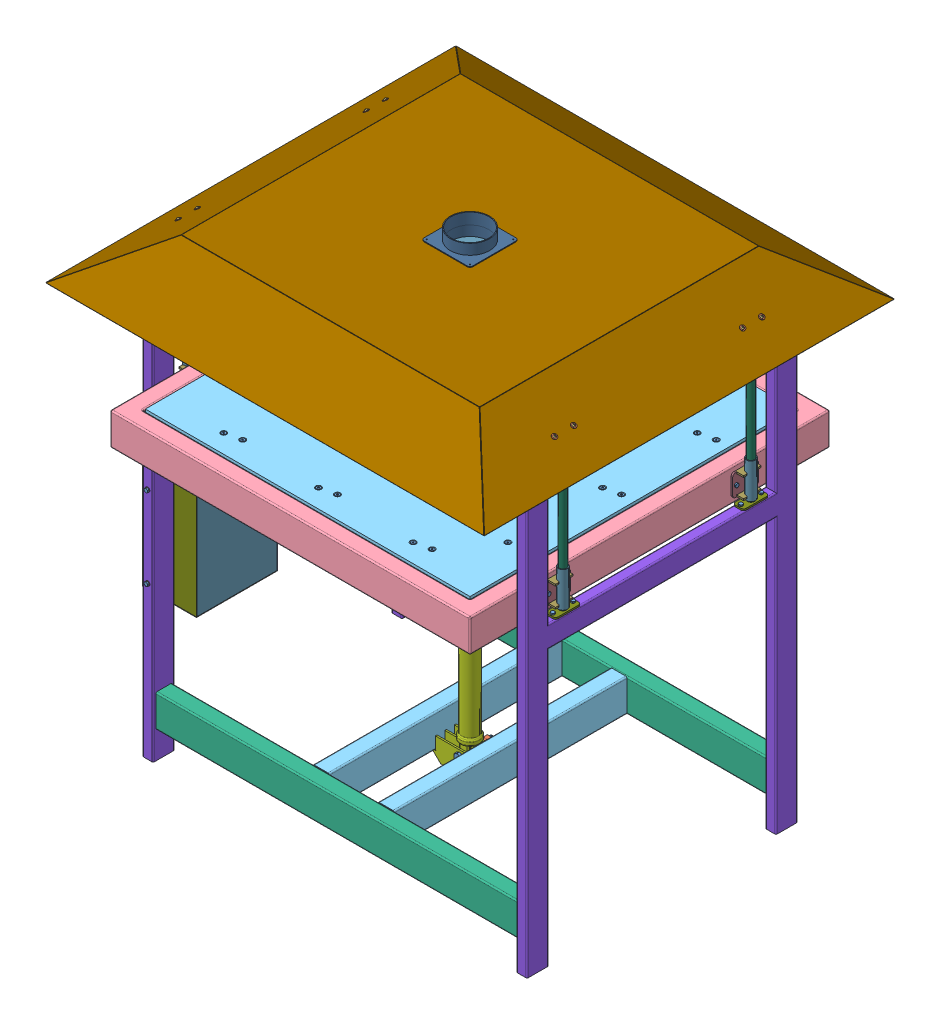
SolidWorks assembly SPR-V1 0000.00-A Sheetpress assembly, configuration Default. Lengths in mm.
Overall size (1624.97 1798.5 1807.96).
665 component instances, 57 part files, 108 mates.
Components (placement in the parent):
- hex bolt gradeab_iso-8: hex bolt gradeab_iso [ISO 4014 - M16 x 120 x 38-S] at (0 -1389 48) x (0 0 -1) z (1 0 0) size (130 27.71 24)
- hex bolt gradeab_iso-10: hex bolt gradeab_iso [ISO 4014 - M16 x 140 x 140-S] at (22.6273 -546.9999 22.6275) x (-0.707107 0 -0.707107) z (0.707107 0 -0.707107) size (150 27.71 24)
- hex nut gradec_iso-137: hex nut gradec_iso [ISO - 4034 - M16 - N] at (0 -1389 -69.8) x (0.923728 0.383049 0) z (0 0 -1) size (24 27.71 15.9)
- hex nut gradec_iso-140: hex nut gradec_iso [ISO - 4034 - M16 - N] at (-65.1246 -546.9999 -65.1245) x (-0.707107 0 0.707107) z (-0.707107 0 -0.707107) size (24 27.71 15.9)
- hex nut gradec_iso-141: hex nut gradec_iso [ISO - 4034 - M16 - N] at (-76.3676 -546.9999 -76.3675) x (-0.707085 -0.007759 0.707085) z (-0.707107 0 -0.707107) size (24 27.71 15.9)
- hex nut gradec_iso-136: hex nut gradec_iso [ISO - 4034 - M16 - N] at (0 -1389 -53.9) x (0.923728 0.383049 0) z (0 0 -1) size (24 27.71 15.9)
- SPR-V1 0000.03-A Spacer-1: SPR-V1 0000.03-A Spacer [Default] at (665 0 0) x (0 0 -1) z (1 0 0) size (40 40 6)
- SPR-V1 0000.03-A Spacer-2: SPR-V1 0000.03-A Spacer [Default] at (671 0 0) x (0 0 1) z (-1 0 0) size (40 40 6)
- SPR-V1 0000.03-A Spacer-3: SPR-V1 0000.03-A Spacer [Default] at (-671 0 0) x (0 0 -1) z (1 0 0) size (40 40 6)
- SPR-V1 0000.03-A Spacer-4: SPR-V1 0000.03-A Spacer [Default] at (-665 0 0) x (0 0 1) z (-1 0 0) size (40 40 6)
- SPR-V1 0000.03-A Spacer-5: SPR-V1 0000.03-A Spacer [Default] at (671 0 -350) x (0 0 1) z (-1 0 0) size (40 40 6)
- SPR-V1 0000.03-A Spacer-6: SPR-V1 0000.03-A Spacer [Default] at (-665 0 -350) x (0 0 1) z (-1 0 0) size (40 40 6)
- plain washer normal grade a_iso-1: plain washer normal grade a_iso [Washer ISO 7089 - 16] at (-711 80 350) size (3 30 30)
- plain washer normal grade a_iso-2: plain washer normal grade a_iso [Washer ISO 7089 - 16] at (-711 80 0) size (3 30 30)
- plain washer normal grade a_iso-3: plain washer normal grade a_iso [Washer ISO 7089 - 16] at (-711 80 -350) size (3 30 30)
- plain washer normal grade a_iso-4: plain washer normal grade a_iso [Washer ISO 7089 - 16] at (605 80 350) size (3 30 30)
- plain washer normal grade a_iso-5: plain washer normal grade a_iso [Washer ISO 7089 - 16] at (605 80 0) size (3 30 30)
- plain washer normal grade a_iso-6: plain washer normal grade a_iso [Washer ISO 7089 - 16] at (605 80 -350) size (3 30 30)
- plain washer normal grade a_iso-7: plain washer normal grade a_iso [Washer ISO 7089 - 16] at (711 80 350) x (-1 0 0) z (0 0.924225 0.381849) size (3 30 30)
- plain washer normal grade a_iso-8: plain washer normal grade a_iso [Washer ISO 7089 - 16] at (711 80 0) x (-1 0 0) z (0 0.924225 0.381849) size (3 30 30)
- plain washer normal grade a_iso-9: plain washer normal grade a_iso [Washer ISO 7089 - 16] at (711 80 -350) x (-1 0 0) z (0 0.924225 0.381849) size (3 30 30)
- plain washer normal grade a_iso-10: plain washer normal grade a_iso [Washer ISO 7089 - 16] at (-605 80 350) x (-1 0 0) z (0 0.924225 0.381849) size (3 30 30)
- plain washer normal grade a_iso-11: plain washer normal grade a_iso [Washer ISO 7089 - 16] at (-605 80 0) x (-1 0 0) z (0 0.924225 0.381849) size (3 30 30)
- plain washer normal grade a_iso-12: plain washer normal grade a_iso [Washer ISO 7089 - 16] at (-605 80 -350) x (-1 0 0) z (0 0.924225 0.381849) size (3 30 30)
- hex bolt gradeab_iso-1: hex bolt gradeab_iso [ISO 4014 - M16 x 140 x 140-S] at (-724 80 350) size (150 27.71 24)
- hex bolt gradeab_iso-2: hex bolt gradeab_iso [ISO 4014 - M16 x 140 x 140-S] at (-724 80 -350) size (150 27.71 24)
- hex bolt gradeab_iso-3: hex bolt gradeab_iso [ISO 4014 - M16 x 140 x 140-S] at (-724 80 0) size (150 27.71 24)
- hex bolt gradeab_iso-4: hex bolt gradeab_iso [ISO 4014 - M16 x 140 x 140-S] at (724 80 -350) x (-1 0 0) z (0 0.924225 0.381849) size (150 27.71 24)
- hex bolt gradeab_iso-5: hex bolt gradeab_iso [ISO 4014 - M16 x 140 x 140-S] at (724 80 0) x (-1 0 0) z (0 0.924225 0.381849) size (150 27.71 24)
- hex bolt gradeab_iso-6: hex bolt gradeab_iso [ISO 4014 - M16 x 140 x 140-S] at (724 80 350) x (-1 0 0) z (0 0.924225 0.381849) size (150 27.71 24)
- hex nut gradec_iso-130: hex nut gradec_iso [ISO - 4034 - M16 - N] at (-586.1 80 -350) x (0 0 -1) z (1 0 0) size (24 27.71 15.9)
- hex nut gradec_iso-131: hex nut gradec_iso [ISO - 4034 - M8 - S] at (-594.1 80 0) x (0 0 -1) z (1 0 0) size (13 15.01 7.9)
- hex nut gradec_iso-132: hex nut gradec_iso [ISO - 4034 - M16 - N] at (-586.1 80 350) x (0 0 -1) z (1 0 0) size (24 27.71 15.9)
- hex nut gradec_iso-133: hex nut gradec_iso [ISO - 4034 - M16 - N] at (586.1 80 350) x (0 0 1) z (-1 0 0) size (24 27.71 15.9)
- hex nut gradec_iso-134: hex nut gradec_iso [ISO - 4034 - M16 - N] at (586.1 80 -350) x (0 0 1) z (-1 0 0) size (24 27.71 15.9)
- hex nut gradec_iso-135: hex nut gradec_iso [ISO - 4034 - M8 - S] at (594.1 80 0) x (0 0 1) z (-1 0 0) size (13 15.01 7.9)
- Frame^SPR-V1 0000.00-A Sheetpress assembly-1: Frame^SPR-V1 0000.00-A Sheetpress assembly [Default] at origin size (1422 1634 1000) (virtual)
  - SPR-V1 0000.01-A Bottom frame jack beams-1: SPR-V1 0000.01-A Bottom frame jack beams [Default] at origin size (300 120 860)
  - SPR-V1 0000.01-A Bottom Frame side beams-1: SPR-V1 0000.01-A Bottom Frame side beams [Default] at (0 0 430) size (1342 120 980)
  - SPR-V1 0000.01-A Jack mount lower-1: SPR-V1 0000.01-A Jack mount lower [Default] at (0 0 35) size (200 80 6)
  - SPR-V1 1000.01-A Side frame-1: SPR-V1 1000.01-A Side frame [Default] at (671 0 0) x (0 0 -1) z (1 0 0) size (1000 1634 40)
  - SPR-V1 1000.01-A Side frame-2: SPR-V1 1000.01-A Side frame [Default] at (-711 0 0) x (0 0 -1) z (1 0 0) size (1000 1634 40)
  - SPR-V1 0000.01-A Jack mount lower-2: SPR-V1 0000.01-A Jack mount lower [Default] at (0 0 -35) size (200 80 6)
  - SPR-V1 0000.01-A Jack mount lower-3: SPR-V1 0000.01-A Jack mount lower [Default] at origin size (200 80 6)
- Pressing plate upper^SPR-V1 0000.00-A Sheetpress assembly-2: Pressing plate upper^SPR-V1 0000.00-A Sheetpress assembly [Default] at origin size (1356.27 127.4 1715) (virtual)
  - SPR-V1 2100.01-A Pressing plate frame upper-1: SPR-V1 2100.01-A Pressing plate frame upper [Default] at origin size (1330 120 1330)
  - SPR-V1 2100.02-A Heating plate upper-1: SPR-V1 2100.02-A Heating plate upper [Default] x (-1 0 0) z (0 -1 0) size (1200 1200 10)
  - SPR-V1 2100.03-A Support structure upper B-1: SPR-V1 2100.03-A Support structure upper B [Default] at (0 107 0) x (-1 0 0) z (0 0 1) size (1210 100 1210)
  - SPR-V1 2100.03-A Pressing plate support structure upper A-1: SPR-V1 2100.03-A Pressing plate support structure upper A [Default] at (0 7 0) size (1210 100 1210)
  - SPR-V1 2100.04-A Sheet mount tabs upper-1: SPR-V1 2100.04-A Sheet mount tabs upper [Default] at (0 118 0) x (-1 0 0) z (0 -1 0) size (46.67 46.67 6.35)
  - SPR-V1 2000.01-A Sheet cover upper-1: SPR-V1 2000.01-A Sheet cover upper [Default] at (0 112 0) x (1 0 0) z (0 1 0) size (1205 1205 1.5)
  - SPR-V1 2100.05-A Suspension plates-1: SPR-V1 2100.05-A Suspension plates [Default] at (260.3787 7 -260.3787) x (0.707107 0 0.707107) z (-0.707107 0 0.707107) size (50 6.43 86)
  - SPR-V1 12 Ceramic terminal-1: SPR-V1 12 Ceramic terminal [Default] at (89.6213 81 89.6213) x (0 -1 0) z (-0.707107 0 0.707107) size (52 24 30)
  - SPR-V1 14 M25 Cable Gland-1: SPR-V1 14 M25 Cable Gland [M20] at (-647.6252 59.9997 552.5039) x (0 0.998679 -0.05138) z (0 0.05138 0.998679) size (33.12 53.02 29.38)
  - SPR-V1 2100.05-A Suspension plates-2: SPR-V1 2100.05-A Suspension plates [Default] at (-260.3787 7 -260.3787) x (0.707107 0 -0.707107) z (0.707107 0 0.707107) size (50 6.43 86)
  - SPR-V1 2100.05-A Suspension plates-3: SPR-V1 2100.05-A Suspension plates [Default] at (-260.3787 7 260.3787) x (-0.707107 0 -0.707107) z (0.707107 0 -0.707107) size (50 6.43 86)
  - SPR-V1 2100.05-A Suspension plates-4: SPR-V1 2100.05-A Suspension plates [Default] at (260.3787 7 260.3787) x (-0.707107 0 0.707107) z (-0.707107 0 -0.707107) size (50 6.43 86)
  - SPR-V1 2000.02-A Heating block-35: SPR-V1 2000.02-A Heating block [Default] at (525.0056 7 524.9944) x (0.707107 0 -0.707107) z (0.707107 0 0.707107) size (50 25 80)
  - SPR-V1 2000.02-A Heating block-32: SPR-V1 2000.02-A Heating block [Default] at (175.0019 7 524.9944) x (0.707107 0 -0.707107) z (0.707107 0 0.707107) size (50 25 80)
  - SPR-V1 2000.02-A Heating block-33: SPR-V1 2000.02-A Heating block [Default] at (350.0037 7 349.9926) x (0.707107 0 -0.707107) z (0.707107 0 0.707107) size (50 25 80)
  - SPR-V1 2000.02-A Heating block-34: SPR-V1 2000.02-A Heating block [Default] at (525.0056 7 174.9907) x (0.707107 0 -0.707107) z (0.707107 0 0.707107) size (50 25 80)
  - SPR-V1 2000.02-A Heating block-44: SPR-V1 2000.02-A Heating block [Default] at (-175.0019 7 524.9944) x (0.707107 0 -0.707107) z (0.707107 0 0.707107) size (50 25 80)
  - SPR-V1 2000.02-A Heating block-45: SPR-V1 2000.02-A Heating block [Default] at (0 7 349.9926) x (0.707107 0 -0.707107) z (0.707107 0 0.707107) size (50 25 80)
  - SPR-V1 2000.02-A Heating block-46: SPR-V1 2000.02-A Heating block [Default] at (175.0019 7 174.9907) x (0.707107 0 -0.707107) z (0.707107 0 0.707107) size (50 25 80)
  - SPR-V1 2000.02-A Heating block-47: SPR-V1 2000.02-A Heating block [Default] at (350.0037 7 -0.0111) x (0.707107 0 -0.707107) z (0.707107 0 0.707107) size (50 25 80)
  - SPR-V1 2000.02-A Heating block-43: SPR-V1 2000.02-A Heating block [Default] at (525.0056 7 -175.013) x (0.707107 0 -0.707107) z (0.707107 0 0.707107) size (50 25 80)
  - SPR-V1 2000.02-A Heating block-36: SPR-V1 2000.02-A Heating block [Default] at (-525.0056 7 524.9944) x (0.707107 0 -0.707107) z (0.707107 0 0.707107) size (50 25 80)
  - SPR-V1 2000.02-A Heating block-37: SPR-V1 2000.02-A Heating block [Default] at (-350.0037 7 349.9926) x (0.707107 0 -0.707107) z (0.707107 0 0.707107) size (50 25 80)
  - SPR-V1 2000.02-A Heating block-42: SPR-V1 2000.02-A Heating block [Default] at (-175.0019 7 174.9907) x (0.707107 0 -0.707107) z (0.707107 0 0.707107) size (50 25 80)
  - SPR-V1 2000.02-A Heating block-38: SPR-V1 2000.02-A Heating block [Default] at (0 7 -0.0111) x (0.707107 0 -0.707107) z (0.707107 0 0.707107) size (50 25 80)
  - SPR-V1 2000.02-A Heating block-40: SPR-V1 2000.02-A Heating block [Default] at (175.0019 7 -175.013) x (0.707107 0 -0.707107) z (0.707107 0 0.707107) size (50 25 80)
  - SPR-V1 2000.02-A Heating block-39: SPR-V1 2000.02-A Heating block [Default] at (350.0037 7 -350.0149) x (0.707107 0 -0.707107) z (0.707107 0 0.707107) size (50 25 80)
  - SPR-V1 2000.02-A Heating block-41: SPR-V1 2000.02-A Heating block [Default] at (525.0056 7 -525.0167) x (0.707107 0 -0.707107) z (0.707107 0 0.707107) size (50 25 80)
  - SPR-V1 2000.02-A Heating block-26: SPR-V1 2000.02-A Heating block [Default] at (-525.0056 7 174.9907) x (0.707107 0 -0.707107) z (0.707107 0 0.707107) size (50 25 80)
  - SPR-V1 2000.02-A Heating block-24: SPR-V1 2000.02-A Heating block [Default] at (-350.0037 7 -0.0111) x (0.707107 0 -0.707107) z (0.707107 0 0.707107) size (50 25 80)
  - SPR-V1 2000.02-A Heating block-27: SPR-V1 2000.02-A Heating block [Default] at (-175.0019 7 -175.013) x (0.707107 0 -0.707107) z (0.707107 0 0.707107) size (50 25 80)
  - SPR-V1 2000.02-A Heating block-29: SPR-V1 2000.02-A Heating block [Default] at (0 7 -350.0149) x (0.707107 0 -0.707107) z (0.707107 0 0.707107) size (50 25 80)
  - SPR-V1 2000.02-A Heating block-30: SPR-V1 2000.02-A Heating block [Default] at (175.0019 7 -525.0167) x (0.707107 0 -0.707107) z (0.707107 0 0.707107) size (50 25 80)
  - SPR-V1 2000.02-A Heating block-31: SPR-V1 2000.02-A Heating block [Default] at (-525.0056 7 -175.013) x (0.707107 0 -0.707107) z (0.707107 0 0.707107) size (50 25 80)
  - SPR-V1 2000.02-A Heating block-23: SPR-V1 2000.02-A Heating block [Default] at (-350.0037 7 -350.0149) x (0.707107 0 -0.707107) z (0.707107 0 0.707107) size (50 25 80)
  - SPR-V1 2000.02-A Heating block-28: SPR-V1 2000.02-A Heating block [Default] at (-175.0019 7 -525.0167) x (0.707107 0 -0.707107) z (0.707107 0 0.707107) size (50 25 80)
  - SPR-V1 2000.02-A Heating block-25: SPR-V1 2000.02-A Heating block [Default] at (-525.0056 7 -525.0167) x (0.707107 0 -0.707107) z (0.707107 0 0.707107) size (50 25 80)
  - SPR-V1 12 Ceramic terminal-2: SPR-V1 12 Ceramic terminal [Default] at (89.6213 81 -89.6213) x (0 -1 0) z (0.707107 0 0.707107) size (52 24 30)
  - SPR-V1 12 Ceramic terminal-3: SPR-V1 12 Ceramic terminal [Default] at (-89.6213 81 -89.6213) x (0 -1 0) z (0.707107 0 -0.707107) size (52 24 30)
  - SPR-V1 12 Ceramic terminal-4: SPR-V1 12 Ceramic terminal [Default] at (-89.6213 81 89.6213) x (0 -1 0) z (-0.707107 0 -0.707107) size (52 24 30)
  - SPR-V1 2100.04-A Sheet mount tabs upper-2: SPR-V1 2100.04-A Sheet mount tabs upper [Default] at (0 118 0) x (0 0 1) z (0 -1 0) size (46.67 46.67 6.35)
  - SPR-V1 2100.04-A Sheet mount tabs upper-3: SPR-V1 2100.04-A Sheet mount tabs upper [Default] at (0 118 0) x (1 0 0) z (0 -1 0) size (46.67 46.67 6.35)
  - SPR-V1 2100.04-A Sheet mount tabs upper-4: SPR-V1 2100.04-A Sheet mount tabs upper [Default] at (0 118 0) x (0 0 -1) z (0 -1 0) size (46.67 46.67 6.35)
  - socket countersunk head screw_iso-1: socket countersunk head screw_iso [ISO 10642 - M8 x 50 - 28N] at (-531.5817 -3 -553.5131) x (0 1 0) z (0 0 1) size (50 15.24 15.24)
  - socket countersunk head screw_iso-2: socket countersunk head screw_iso [ISO 10642 - M8 x 50 - 28N] at (-181.578 -3 -553.5131) x (0 1 0) z (0 0 1) size (50 15.24 15.24)
  - socket countersunk head screw_iso-3: socket countersunk head screw_iso [ISO 10642 - M8 x 50 - 28N] at (-356.5798 -3 -378.5113) x (0 1 0) z (0 0 1) size (50 15.24 15.24)
  - socket countersunk head screw_iso-4: socket countersunk head screw_iso [ISO 10642 - M8 x 50 - 28N] at (-531.5817 -3 -203.5094) x (0 1 0) z (0 0 1) size (50 15.24 15.24)
  - socket countersunk head screw_iso-5: socket countersunk head screw_iso [ISO 10642 - M8 x 50 - 28N] at (168.4258 -3 -553.5131) x (0 1 0) z (0 0 1) size (50 15.24 15.24)
  - socket countersunk head screw_iso-6: socket countersunk head screw_iso [ISO 10642 - M8 x 50 - 28N] at (-6.5761 -3 -378.5113) x (0 1 0) z (0 0 1) size (50 15.24 15.24)
  - socket countersunk head screw_iso-7: socket countersunk head screw_iso [ISO 10642 - M8 x 50 - 28N] at (-181.578 -3 -203.5094) x (0 1 0) z (0 0 1) size (50 15.24 15.24)
  - socket countersunk head screw_iso-8: socket countersunk head screw_iso [ISO 10642 - M8 x 50 - 28N] at (-356.5798 -3 -28.5075) x (0 1 0) z (0 0 1) size (50 15.24 15.24)
  - socket countersunk head screw_iso-9: socket countersunk head screw_iso [ISO 10642 - M8 x 50 - 28N] at (-531.5817 -3 146.4943) x (0 1 0) z (0 0 1) size (50 15.24 15.24)
  - socket countersunk head screw_iso-10: socket countersunk head screw_iso [ISO 10642 - M8 x 50 - 28N] at (518.4295 -3 -553.5131) x (0 1 0) z (0 0 1) size (50 15.24 15.24)
  - socket countersunk head screw_iso-11: socket countersunk head screw_iso [ISO 10642 - M8 x 50 - 28N] at (343.4276 -3 -378.5113) x (0 1 0) z (0 0 1) size (50 15.24 15.24)
  - socket countersunk head screw_iso-12: socket countersunk head screw_iso [ISO 10642 - M8 x 50 - 28N] at (168.4258 -3 -203.5094) x (0 1 0) z (0 0 1) size (50 15.24 15.24)
  - socket countersunk head screw_iso-13: socket countersunk head screw_iso [ISO 10642 - M8 x 50 - 28N] at (-6.5761 -3 -28.5075) x (0 1 0) z (0 0 1) size (50 15.24 15.24)
  - socket countersunk head screw_iso-14: socket countersunk head screw_iso [ISO 10642 - M8 x 50 - 28N] at (-181.578 -3 146.4943) x (0 1 0) z (0 0 1) size (50 15.24 15.24)
  - socket countersunk head screw_iso-15: socket countersunk head screw_iso [ISO 10642 - M8 x 50 - 28N] at (-356.5798 -3 321.4962) x (0 1 0) z (0 0 1) size (50 15.24 15.24)
  - socket countersunk head screw_iso-16: socket countersunk head screw_iso [ISO 10642 - M8 x 50 - 28N] at (-531.5817 -3 496.498) x (0 1 0) z (0 0 1) size (50 15.24 15.24)
  - socket countersunk head screw_iso-17: socket countersunk head screw_iso [ISO 10642 - M8 x 50 - 28N] at (518.4295 -3 -203.5094) x (0 1 0) z (0 0 1) size (50 15.24 15.24)
  - socket countersunk head screw_iso-18: socket countersunk head screw_iso [ISO 10642 - M8 x 50 - 28N] at (343.4276 -3 -28.5075) x (0 1 0) z (0 0 1) size (50 15.24 15.24)
  - socket countersunk head screw_iso-19: socket countersunk head screw_iso [ISO 10642 - M8 x 50 - 28N] at (168.4258 -3 146.4943) x (0 1 0) z (0 0 1) size (50 15.24 15.24)
  - socket countersunk head screw_iso-20: socket countersunk head screw_iso [ISO 10642 - M8 x 50 - 28N] at (-6.5761 -3 321.4962) x (0 1 0) z (0 0 1) size (50 15.24 15.24)
  - socket countersunk head screw_iso-21: socket countersunk head screw_iso [ISO 10642 - M8 x 50 - 28N] at (-181.578 -3 496.498) x (0 1 0) z (0 0 1) size (50 15.24 15.24)
  - socket countersunk head screw_iso-22: socket countersunk head screw_iso [ISO 10642 - M8 x 50 - 28N] at (518.4295 -3 146.4943) x (0 1 0) z (0 0 1) size (50 15.24 15.24)
  - socket countersunk head screw_iso-23: socket countersunk head screw_iso [ISO 10642 - M8 x 50 - 28N] at (343.4276 -3 321.4962) x (0 1 0) z (0 0 1) size (50 15.24 15.24)
  - socket countersunk head screw_iso-24: socket countersunk head screw_iso [ISO 10642 - M8 x 50 - 28N] at (168.4258 -3 496.498) x (0 1 0) z (0 0 1) size (50 15.24 15.24)
  - socket countersunk head screw_iso-25: socket countersunk head screw_iso [ISO 10642 - M8 x 50 - 28N] at (518.4295 -3 496.498) x (0 1 0) z (0 0 1) size (50 15.24 15.24)
  - socket countersunk head screw_iso-26: socket countersunk head screw_iso [ISO 10642 - M8 x 50 - 28N] at (-518.4295 -3 -496.5203) x (0 1 0) z (-0.546944 0 0.837169) size (50 15.24 15.24)
  - socket countersunk head screw_iso-27: socket countersunk head screw_iso [ISO 10642 - M8 x 50 - 28N] at (-168.4258 -3 -496.5203) x (0 1 0) z (-0.546944 0 0.837169) size (50 15.24 15.24)
  - socket countersunk head screw_iso-28: socket countersunk head screw_iso [ISO 10642 - M8 x 50 - 28N] at (-343.4276 -3 -321.5185) x (0 1 0) z (-0.546944 0 0.837169) size (50 15.24 15.24)
  - socket countersunk head screw_iso-29: socket countersunk head screw_iso [ISO 10642 - M8 x 50 - 28N] at (-518.4295 -3 -146.5166) x (0 1 0) z (-0.546944 0 0.837169) size (50 15.24 15.24)
  - socket countersunk head screw_iso-30: socket countersunk head screw_iso [ISO 10642 - M8 x 50 - 28N] at (181.578 -3 -496.5203) x (0 1 0) z (-0.546944 0 0.837169) size (50 15.24 15.24)
  - socket countersunk head screw_iso-31: socket countersunk head screw_iso [ISO 10642 - M8 x 50 - 28N] at (6.5761 -3 -321.5185) x (0 1 0) z (-0.546944 0 0.837169) size (50 15.24 15.24)
  - socket countersunk head screw_iso-32: socket countersunk head screw_iso [ISO 10642 - M8 x 50 - 28N] at (-168.4258 -3 -146.5166) x (0 1 0) z (-0.546944 0 0.837169) size (50 15.24 15.24)
  - socket countersunk head screw_iso-33: socket countersunk head screw_iso [ISO 10642 - M8 x 50 - 28N] at (-343.4276 -3 28.4853) x (0 1 0) z (-0.546944 0 0.837169) size (50 15.24 15.24)
  - socket countersunk head screw_iso-34: socket countersunk head screw_iso [ISO 10642 - M8 x 50 - 28N] at (-518.4295 -3 203.4871) x (0 1 0) z (-0.546944 0 0.837169) size (50 15.24 15.24)
  - socket countersunk head screw_iso-35: socket countersunk head screw_iso [ISO 10642 - M8 x 50 - 28N] at (531.5817 -3 -496.5203) x (0 1 0) z (-0.546944 0 0.837169) size (50 15.24 15.24)
  - socket countersunk head screw_iso-36: socket countersunk head screw_iso [ISO 10642 - M8 x 50 - 28N] at (356.5798 -3 -321.5185) x (0 1 0) z (-0.546944 0 0.837169) size (50 15.24 15.24)
  - socket countersunk head screw_iso-37: socket countersunk head screw_iso [ISO 10642 - M8 x 50 - 28N] at (181.578 -3 -146.5166) x (0 1 0) z (-0.546944 0 0.837169) size (50 15.24 15.24)
  - socket countersunk head screw_iso-38: socket countersunk head screw_iso [ISO 10642 - M8 x 50 - 28N] at (6.5761 -3 28.4853) x (0 1 0) z (-0.546944 0 0.837169) size (50 15.24 15.24)
  - socket countersunk head screw_iso-39: socket countersunk head screw_iso [ISO 10642 - M8 x 50 - 28N] at (-168.4258 -3 203.4871) x (0 1 0) z (-0.546944 0 0.837169) size (50 15.24 15.24)
  - socket countersunk head screw_iso-40: socket countersunk head screw_iso [ISO 10642 - M8 x 50 - 28N] at (-343.4276 -3 378.489) x (0 1 0) z (-0.546944 0 0.837169) size (50 15.24 15.24)
  - socket countersunk head screw_iso-41: socket countersunk head screw_iso [ISO 10642 - M8 x 50 - 28N] at (-518.4295 -3 553.4908) x (0 1 0) z (-0.546944 0 0.837169) size (50 15.24 15.24)
  - socket countersunk head screw_iso-42: socket countersunk head screw_iso [ISO 10642 - M8 x 50 - 28N] at (531.5817 -3 -146.5166) x (0 1 0) z (-0.546944 0 0.837169) size (50 15.24 15.24)
  - socket countersunk head screw_iso-43: socket countersunk head screw_iso [ISO 10642 - M8 x 50 - 28N] at (356.5798 -3 28.4853) x (0 1 0) z (-0.546944 0 0.837169) size (50 15.24 15.24)
  - socket countersunk head screw_iso-44: socket countersunk head screw_iso [ISO 10642 - M8 x 50 - 28N] at (181.578 -3 203.4871) x (0 1 0) z (-0.546944 0 0.837169) size (50 15.24 15.24)
  - socket countersunk head screw_iso-45: socket countersunk head screw_iso [ISO 10642 - M8 x 50 - 28N] at (6.5761 -3 378.489) x (0 1 0) z (-0.546944 0 0.837169) size (50 15.24 15.24)
  - socket countersunk head screw_iso-46: socket countersunk head screw_iso [ISO 10642 - M8 x 50 - 28N] at (-168.4258 -3 553.4908) x (0 1 0) z (-0.546944 0 0.837169) size (50 15.24 15.24)
  - socket countersunk head screw_iso-47: socket countersunk head screw_iso [ISO 10642 - M8 x 50 - 28N] at (531.5817 -3 203.4871) x (0 1 0) z (-0.546944 0 0.837169) size (50 15.24 15.24)
  - socket countersunk head screw_iso-48: socket countersunk head screw_iso [ISO 10642 - M8 x 50 - 28N] at (356.5798 -3 378.489) x (0 1 0) z (-0.546944 0 0.837169) size (50 15.24 15.24)
  - socket countersunk head screw_iso-49: socket countersunk head screw_iso [ISO 10642 - M8 x 50 - 28N] at (181.578 -3 553.4908) x (0 1 0) z (-0.546944 0 0.837169) size (50 15.24 15.24)
  - socket countersunk head screw_iso-50: socket countersunk head screw_iso [ISO 10642 - M8 x 50 - 28N] at (531.5817 -3 553.4908) x (0 1 0) z (-0.546944 0 0.837169) size (50 15.24 15.24)
  - plain washer normal grade a_iso-1: plain washer normal grade a_iso [Washer ISO 7089 - 8] at (-531.5817 32 -553.5131) x (0 -1 0) z (0 0 1) size (1.6 16 16)
  - plain washer normal grade a_iso-2: plain washer normal grade a_iso [Washer ISO 7089 - 8] at (-181.578 32 -553.5131) x (0 -1 0) z (0 0 1) size (1.6 16 16)
  - plain washer normal grade a_iso-3: plain washer normal grade a_iso [Washer ISO 7089 - 8] at (-356.5798 32 -378.5113) x (0 -1 0) z (0 0 1) size (1.6 16 16)
  - plain washer normal grade a_iso-4: plain washer normal grade a_iso [Washer ISO 7089 - 8] at (-531.5817 32 -203.5094) x (0 -1 0) z (0 0 1) size (1.6 16 16)
  - plain washer normal grade a_iso-5: plain washer normal grade a_iso [Washer ISO 7089 - 8] at (168.4258 32 -553.5131) x (0 -1 0) z (0 0 1) size (1.6 16 16)
  - plain washer normal grade a_iso-6: plain washer normal grade a_iso [Washer ISO 7089 - 8] at (-6.5761 32 -378.5113) x (0 -1 0) z (0 0 1) size (1.6 16 16)
  - plain washer normal grade a_iso-7: plain washer normal grade a_iso [Washer ISO 7089 - 8] at (-181.578 32 -203.5094) x (0 -1 0) z (0 0 1) size (1.6 16 16)
  - plain washer normal grade a_iso-8: plain washer normal grade a_iso [Washer ISO 7089 - 8] at (-356.5798 32 -28.5075) x (0 -1 0) z (0 0 1) size (1.6 16 16)
  - plain washer normal grade a_iso-9: plain washer normal grade a_iso [Washer ISO 7089 - 8] at (-531.5817 32 146.4943) x (0 -1 0) z (0 0 1) size (1.6 16 16)
  - plain washer normal grade a_iso-10: plain washer normal grade a_iso [Washer ISO 7089 - 8] at (518.4295 32 -553.5131) x (0 -1 0) z (0 0 1) size (1.6 16 16)
  - plain washer normal grade a_iso-11: plain washer normal grade a_iso [Washer ISO 7089 - 8] at (343.4276 32 -378.5113) x (0 -1 0) z (0 0 1) size (1.6 16 16)
  - plain washer normal grade a_iso-12: plain washer normal grade a_iso [Washer ISO 7089 - 8] at (168.4258 32 -203.5094) x (0 -1 0) z (0 0 1) size (1.6 16 16)
  - plain washer normal grade a_iso-13: plain washer normal grade a_iso [Washer ISO 7089 - 8] at (-6.5761 32 -28.5075) x (0 -1 0) z (0 0 1) size (1.6 16 16)
  - plain washer normal grade a_iso-14: plain washer normal grade a_iso [Washer ISO 7089 - 8] at (-181.578 32 146.4943) x (0 -1 0) z (0 0 1) size (1.6 16 16)
  - plain washer normal grade a_iso-15: plain washer normal grade a_iso [Washer ISO 7089 - 8] at (-356.5798 32 321.4962) x (0 -1 0) z (0 0 1) size (1.6 16 16)
  - plain washer normal grade a_iso-16: plain washer normal grade a_iso [Washer ISO 7089 - 8] at (-531.5817 32 496.498) x (0 -1 0) z (0 0 1) size (1.6 16 16)
  - plain washer normal grade a_iso-17: plain washer normal grade a_iso [Washer ISO 7089 - 8] at (518.4295 32 -203.5094) x (0 -1 0) z (0 0 1) size (1.6 16 16)
  - plain washer normal grade a_iso-18: plain washer normal grade a_iso [Washer ISO 7089 - 8] at (343.4276 32 -28.5075) x (0 -1 0) z (0 0 1) size (1.6 16 16)
  - plain washer normal grade a_iso-19: plain washer normal grade a_iso [Washer ISO 7089 - 8] at (168.4258 32 146.4943) x (0 -1 0) z (0 0 1) size (1.6 16 16)
  - plain washer normal grade a_iso-20: plain washer normal grade a_iso [Washer ISO 7089 - 8] at (-6.5761 32 321.4962) x (0 -1 0) z (0 0 1) size (1.6 16 16)
  - plain washer normal grade a_iso-21: plain washer normal grade a_iso [Washer ISO 7089 - 8] at (-181.578 32 496.498) x (0 -1 0) z (0 0 1) size (1.6 16 16)
  - plain washer normal grade a_iso-22: plain washer normal grade a_iso [Washer ISO 7089 - 8] at (518.4295 32 146.4943) x (0 -1 0) z (0 0 1) size (1.6 16 16)
  - plain washer normal grade a_iso-23: plain washer normal grade a_iso [Washer ISO 7089 - 8] at (343.4276 32 321.4962) x (0 -1 0) z (0 0 1) size (1.6 16 16)
  - plain washer normal grade a_iso-24: plain washer normal grade a_iso [Washer ISO 7089 - 8] at (168.4258 32 496.498) x (0 -1 0) z (0 0 1) size (1.6 16 16)
  - plain washer normal grade a_iso-25: plain washer normal grade a_iso [Washer ISO 7089 - 8] at (518.4295 32 496.498) x (0 -1 0) z (0 0 1) size (1.6 16 16)
  - plain washer normal grade a_iso-26: plain washer normal grade a_iso [Washer ISO 7089 - 8] at (-518.4295 32 -496.5203) x (0 -1 0) z (0 0 1) size (1.6 16 16)
  - plain washer normal grade a_iso-27: plain washer normal grade a_iso [Washer ISO 7089 - 8] at (-168.4258 32 -496.5203) x (0 -1 0) z (0 0 1) size (1.6 16 16)
  - plain washer normal grade a_iso-28: plain washer normal grade a_iso [Washer ISO 7089 - 8] at (-343.4276 32 -321.5185) x (0 -1 0) z (0 0 1) size (1.6 16 16)
  - plain washer normal grade a_iso-29: plain washer normal grade a_iso [Washer ISO 7089 - 8] at (-518.4295 32 -146.5166) x (0 -1 0) z (0 0 1) size (1.6 16 16)
  - plain washer normal grade a_iso-30: plain washer normal grade a_iso [Washer ISO 7089 - 8] at (181.578 32 -496.5203) x (0 -1 0) z (0 0 1) size (1.6 16 16)
  - plain washer normal grade a_iso-31: plain washer normal grade a_iso [Washer ISO 7089 - 8] at (6.5761 32 -321.5185) x (0 -1 0) z (0 0 1) size (1.6 16 16)
  - plain washer normal grade a_iso-32: plain washer normal grade a_iso [Washer ISO 7089 - 8] at (-168.4258 32 -146.5166) x (0 -1 0) z (0 0 1) size (1.6 16 16)
  - plain washer normal grade a_iso-33: plain washer normal grade a_iso [Washer ISO 7089 - 8] at (-343.4276 32 28.4853) x (0 -1 0) z (0 0 1) size (1.6 16 16)
  - plain washer normal grade a_iso-34: plain washer normal grade a_iso [Washer ISO 7089 - 8] at (-518.4295 32 203.4871) x (0 -1 0) z (0 0 1) size (1.6 16 16)
  - plain washer normal grade a_iso-35: plain washer normal grade a_iso [Washer ISO 7089 - 8] at (531.5817 32 -496.5203) x (0 -1 0) z (0 0 1) size (1.6 16 16)
  - plain washer normal grade a_iso-36: plain washer normal grade a_iso [Washer ISO 7089 - 8] at (356.5798 32 -321.5185) x (0 -1 0) z (0 0 1) size (1.6 16 16)
  - plain washer normal grade a_iso-37: plain washer normal grade a_iso [Washer ISO 7089 - 8] at (181.578 32 -146.5166) x (0 -1 0) z (0 0 1) size (1.6 16 16)
  - plain washer normal grade a_iso-38: plain washer normal grade a_iso [Washer ISO 7089 - 8] at (6.5761 32 28.4853) x (0 -1 0) z (0 0 1) size (1.6 16 16)
  - plain washer normal grade a_iso-39: plain washer normal grade a_iso [Washer ISO 7089 - 8] at (-168.4258 32 203.4871) x (0 -1 0) z (0 0 1) size (1.6 16 16)
  - plain washer normal grade a_iso-40: plain washer normal grade a_iso [Washer ISO 7089 - 8] at (-343.4276 32 378.489) x (0 -1 0) z (0 0 1) size (1.6 16 16)
  - plain washer normal grade a_iso-41: plain washer normal grade a_iso [Washer ISO 7089 - 8] at (-518.4295 32 553.4908) x (0 -1 0) z (0 0 1) size (1.6 16 16)
  - plain washer normal grade a_iso-42: plain washer normal grade a_iso [Washer ISO 7089 - 8] at (531.5817 32 -146.5166) x (0 -1 0) z (0 0 1) size (1.6 16 16)
  - plain washer normal grade a_iso-43: plain washer normal grade a_iso [Washer ISO 7089 - 8] at (356.5798 32 28.4853) x (0 -1 0) z (0 0 1) size (1.6 16 16)
  - plain washer normal grade a_iso-44: plain washer normal grade a_iso [Washer ISO 7089 - 8] at (181.578 32 203.4871) x (0 -1 0) z (0 0 1) size (1.6 16 16)
  - plain washer normal grade a_iso-45: plain washer normal grade a_iso [Washer ISO 7089 - 8] at (6.5761 32 378.489) x (0 -1 0) z (0 0 1) size (1.6 16 16)
  - plain washer normal grade a_iso-46: plain washer normal grade a_iso [Washer ISO 7089 - 8] at (-168.4258 32 553.4908) x (0 -1 0) z (0 0 1) size (1.6 16 16)
  - plain washer normal grade a_iso-47: plain washer normal grade a_iso [Washer ISO 7089 - 8] at (531.5817 32 203.4871) x (0 -1 0) z (0 0 1) size (1.6 16 16)
  - plain washer normal grade a_iso-48: plain washer normal grade a_iso [Washer ISO 7089 - 8] at (356.5798 32 378.489) x (0 -1 0) z (0 0 1) size (1.6 16 16)
  - plain washer normal grade a_iso-49: plain washer normal grade a_iso [Washer ISO 7089 - 8] at (181.578 32 553.4908) x (0 -1 0) z (0 0 1) size (1.6 16 16)
  - plain washer normal grade a_iso-50: plain washer normal grade a_iso [Washer ISO 7089 - 8] at (531.5817 32 553.4908) x (0 -1 0) z (0 0 1) size (1.6 16 16)
  - hex nut gradec_iso-1: hex nut gradec_iso [ISO - 4034 - M8 - N] at (-531.5817 41.5 -553.5131) x (1 0 0) z (0 1 0) size (13 15.01 7.9)
  - hex nut gradec_iso-2: hex nut gradec_iso [ISO - 4034 - M8 - N] at (-181.578 41.5 -553.5131) x (1 0 0) z (0 1 0) size (13 15.01 7.9)
  - hex nut gradec_iso-3: hex nut gradec_iso [ISO - 4034 - M8 - N] at (-356.5798 41.5 -378.5113) x (1 0 0) z (0 1 0) size (13 15.01 7.9)
  - hex nut gradec_iso-4: hex nut gradec_iso [ISO - 4034 - M8 - N] at (-531.5817 41.5 -203.5094) x (1 0 0) z (0 1 0) size (13 15.01 7.9)
  - hex nut gradec_iso-5: hex nut gradec_iso [ISO - 4034 - M8 - N] at (168.4258 41.5 -553.5131) x (1 0 0) z (0 1 0) size (13 15.01 7.9)
  - hex nut gradec_iso-6: hex nut gradec_iso [ISO - 4034 - M8 - N] at (-6.5761 41.5 -378.5113) x (1 0 0) z (0 1 0) size (13 15.01 7.9)
  - hex nut gradec_iso-7: hex nut gradec_iso [ISO - 4034 - M8 - N] at (-181.578 41.5 -203.5094) x (1 0 0) z (0 1 0) size (13 15.01 7.9)
  - hex nut gradec_iso-8: hex nut gradec_iso [ISO - 4034 - M8 - N] at (-356.5798 41.5 -28.5075) x (1 0 0) z (0 1 0) size (13 15.01 7.9)
  - hex nut gradec_iso-9: hex nut gradec_iso [ISO - 4034 - M8 - N] at (-531.5817 41.5 146.4943) x (1 0 0) z (0 1 0) size (13 15.01 7.9)
  - hex nut gradec_iso-10: hex nut gradec_iso [ISO - 4034 - M8 - N] at (518.4295 41.5 -553.5131) x (1 0 0) z (0 1 0) size (13 15.01 7.9)
  - hex nut gradec_iso-11: hex nut gradec_iso [ISO - 4034 - M8 - N] at (343.4276 41.5 -378.5113) x (1 0 0) z (0 1 0) size (13 15.01 7.9)
  - hex nut gradec_iso-12: hex nut gradec_iso [ISO - 4034 - M8 - N] at (168.4258 41.5 -203.5094) x (1 0 0) z (0 1 0) size (13 15.01 7.9)
  - hex nut gradec_iso-13: hex nut gradec_iso [ISO - 4034 - M8 - N] at (-6.5761 41.5 -28.5075) x (1 0 0) z (0 1 0) size (13 15.01 7.9)
  - hex nut gradec_iso-14: hex nut gradec_iso [ISO - 4034 - M8 - N] at (-181.578 41.5 146.4943) x (1 0 0) z (0 1 0) size (13 15.01 7.9)
  - hex nut gradec_iso-15: hex nut gradec_iso [ISO - 4034 - M8 - N] at (-356.5798 41.5 321.4962) x (1 0 0) z (0 1 0) size (13 15.01 7.9)
  - hex nut gradec_iso-16: hex nut gradec_iso [ISO - 4034 - M8 - N] at (-531.5817 41.5 496.498) x (1 0 0) z (0 1 0) size (13 15.01 7.9)
  - hex nut gradec_iso-17: hex nut gradec_iso [ISO - 4034 - M8 - N] at (518.4295 41.5 -203.5094) x (1 0 0) z (0 1 0) size (13 15.01 7.9)
  - hex nut gradec_iso-18: hex nut gradec_iso [ISO - 4034 - M8 - N] at (343.4276 41.5 -28.5075) x (1 0 0) z (0 1 0) size (13 15.01 7.9)
  - hex nut gradec_iso-19: hex nut gradec_iso [ISO - 4034 - M8 - N] at (168.4258 41.5 146.4943) x (1 0 0) z (0 1 0) size (13 15.01 7.9)
  - hex nut gradec_iso-20: hex nut gradec_iso [ISO - 4034 - M8 - N] at (-6.5761 41.5 321.4962) x (1 0 0) z (0 1 0) size (13 15.01 7.9)
  - hex nut gradec_iso-21: hex nut gradec_iso [ISO - 4034 - M8 - N] at (-181.578 41.5 496.498) x (1 0 0) z (0 1 0) size (13 15.01 7.9)
  - hex nut gradec_iso-22: hex nut gradec_iso [ISO - 4034 - M8 - N] at (518.4295 41.5 146.4943) x (1 0 0) z (0 1 0) size (13 15.01 7.9)
  - hex nut gradec_iso-23: hex nut gradec_iso [ISO - 4034 - M8 - N] at (343.4276 41.5 321.4962) x (1 0 0) z (0 1 0) size (13 15.01 7.9)
  - hex nut gradec_iso-24: hex nut gradec_iso [ISO - 4034 - M8 - N] at (168.4258 41.5 496.498) x (1 0 0) z (0 1 0) size (13 15.01 7.9)
  - hex nut gradec_iso-25: hex nut gradec_iso [ISO - 4034 - M8 - N] at (518.4295 41.5 496.498) x (1 0 0) z (0 1 0) size (13 15.01 7.9)
  - hex nut gradec_iso-26: hex nut gradec_iso [ISO - 4034 - M8 - N] at (-518.4295 41.5 -496.5203) x (1 0 0) z (0 1 0) size (13 15.01 7.9)
  - hex nut gradec_iso-27: hex nut gradec_iso [ISO - 4034 - M8 - N] at (-168.4258 41.5 -496.5203) x (1 0 0) z (0 1 0) size (13 15.01 7.9)
  - hex nut gradec_iso-28: hex nut gradec_iso [ISO - 4034 - M8 - N] at (-343.4276 41.5 -321.5185) x (1 0 0) z (0 1 0) size (13 15.01 7.9)
  - hex nut gradec_iso-29: hex nut gradec_iso [ISO - 4034 - M8 - N] at (-518.4295 41.5 -146.5166) x (1 0 0) z (0 1 0) size (13 15.01 7.9)
  - hex nut gradec_iso-30: hex nut gradec_iso [ISO - 4034 - M8 - N] at (181.578 41.5 -496.5203) x (1 0 0) z (0 1 0) size (13 15.01 7.9)
  - hex nut gradec_iso-31: hex nut gradec_iso [ISO - 4034 - M8 - N] at (6.5761 41.5 -321.5185) x (1 0 0) z (0 1 0) size (13 15.01 7.9)
  - hex nut gradec_iso-32: hex nut gradec_iso [ISO - 4034 - M8 - N] at (-168.4258 41.5 -146.5166) x (1 0 0) z (0 1 0) size (13 15.01 7.9)
  - hex nut gradec_iso-33: hex nut gradec_iso [ISO - 4034 - M8 - N] at (-343.4276 41.5 28.4853) x (1 0 0) z (0 1 0) size (13 15.01 7.9)
  - hex nut gradec_iso-34: hex nut gradec_iso [ISO - 4034 - M8 - N] at (-518.4295 41.5 203.4871) x (1 0 0) z (0 1 0) size (13 15.01 7.9)
  - hex nut gradec_iso-35: hex nut gradec_iso [ISO - 4034 - M8 - N] at (531.5817 41.5 -496.5203) x (1 0 0) z (0 1 0) size (13 15.01 7.9)
  - hex nut gradec_iso-36: hex nut gradec_iso [ISO - 4034 - M8 - N] at (356.5798 41.5 -321.5185) x (1 0 0) z (0 1 0) size (13 15.01 7.9)
  - hex nut gradec_iso-37: hex nut gradec_iso [ISO - 4034 - M8 - N] at (181.578 41.5 -146.5166) x (1 0 0) z (0 1 0) size (13 15.01 7.9)
  - hex nut gradec_iso-38: hex nut gradec_iso [ISO - 4034 - M8 - N] at (6.5761 41.5 28.4853) x (1 0 0) z (0 1 0) size (13 15.01 7.9)
  - hex nut gradec_iso-39: hex nut gradec_iso [ISO - 4034 - M8 - N] at (-168.4258 41.5 203.4871) x (1 0 0) z (0 1 0) size (13 15.01 7.9)
  - hex nut gradec_iso-40: hex nut gradec_iso [ISO - 4034 - M8 - N] at (-343.4276 41.5 378.489) x (1 0 0) z (0 1 0) size (13 15.01 7.9)
  - hex nut gradec_iso-41: hex nut gradec_iso [ISO - 4034 - M8 - N] at (-518.4295 41.5 553.4908) x (1 0 0) z (0 1 0) size (13 15.01 7.9)
  - hex nut gradec_iso-42: hex nut gradec_iso [ISO - 4034 - M8 - N] at (531.5817 41.5 -146.5166) x (1 0 0) z (0 1 0) size (13 15.01 7.9)
  - hex nut gradec_iso-43: hex nut gradec_iso [ISO - 4034 - M8 - N] at (356.5798 41.5 28.4853) x (1 0 0) z (0 1 0) size (13 15.01 7.9)
  - hex nut gradec_iso-44: hex nut gradec_iso [ISO - 4034 - M8 - N] at (181.578 41.5 203.4871) x (1 0 0) z (0 1 0) size (13 15.01 7.9)
  - hex nut gradec_iso-45: hex nut gradec_iso [ISO - 4034 - M8 - N] at (6.5761 41.5 378.489) x (1 0 0) z (0 1 0) size (13 15.01 7.9)
  - hex nut gradec_iso-46: hex nut gradec_iso [ISO - 4034 - M8 - N] at (-168.4258 41.5 553.4908) x (1 0 0) z (0 1 0) size (13 15.01 7.9)
  - hex nut gradec_iso-47: hex nut gradec_iso [ISO - 4034 - M8 - N] at (531.5817 41.5 203.4871) x (1 0 0) z (0 1 0) size (13 15.01 7.9)
  - hex nut gradec_iso-48: hex nut gradec_iso [ISO - 4034 - M8 - N] at (356.5798 41.5 378.489) x (1 0 0) z (0 1 0) size (13 15.01 7.9)
  - hex nut gradec_iso-49: hex nut gradec_iso [ISO - 4034 - M8 - N] at (181.578 41.5 553.4908) x (1 0 0) z (0 1 0) size (13 15.01 7.9)
  - hex nut gradec_iso-50: hex nut gradec_iso [ISO - 4034 - M8 - N] at (531.5817 41.5 553.4908) x (1 0 0) z (0 1 0) size (13 15.01 7.9)
  - socket countersunk head screw_iso-51: socket countersunk head screw_iso [ISO 10642 - M8 x 50 - 28N] at (-278.7769 -3 278.75) x (0 1 0) z (1 0 0) size (50 15.24 15.24)
  - socket countersunk head screw_iso-52: socket countersunk head screw_iso [ISO 10642 - M8 x 50 - 28N] at (-278.75 -3 -278.7769) x (0 1 0) z (0 0 1) size (50 15.24 15.24)
  - socket countersunk head screw_iso-53: socket countersunk head screw_iso [ISO 10642 - M8 x 50 - 28N] at (278.7769 -3 -278.75) x (0 1 0) z (-1 0 0) size (50 15.24 15.24)
  - socket countersunk head screw_iso-54: socket countersunk head screw_iso [ISO 10642 - M8 x 50 - 28N] at (278.75 -3 278.7769) x (0 1 0) z (0 0 -1) size (50 15.24 15.24)
  - socket countersunk head screw_iso-55: socket countersunk head screw_iso [ISO 10642 - M8 x 50 - 28N] at (-246.25 -3 246.2231) x (0 1 0) z (1 0 0) size (50 15.24 15.24)
  - socket countersunk head screw_iso-56: socket countersunk head screw_iso [ISO 10642 - M8 x 50 - 28N] at (-246.2231 -3 -246.25) x (0 1 0) z (0 0 1) size (50 15.24 15.24)
  - socket countersunk head screw_iso-57: socket countersunk head screw_iso [ISO 10642 - M8 x 50 - 28N] at (246.25 -3 -246.2231) x (0 1 0) z (-1 0 0) size (50 15.24 15.24)
  - socket countersunk head screw_iso-58: socket countersunk head screw_iso [ISO 10642 - M8 x 50 - 28N] at (246.2231 -3 246.25) x (0 1 0) z (0 0 -1) size (50 15.24 15.24)
  - hex nut gradec_iso-51: hex nut gradec_iso [ISO - 4034 - M8 - N] at (278.75 39.9 278.7769) x (1 0 0) z (0 1 0) size (13 15.01 7.9)
  - hex nut gradec_iso-52: hex nut gradec_iso [ISO - 4034 - M8 - N] at (246.2231 39.9 246.25) x (1 0 0) z (0 1 0) size (13 15.01 7.9)
  - hex nut gradec_iso-53: hex nut gradec_iso [ISO - 4034 - M8 - N] at (-278.7769 39.9 278.75) x (1 0 0) z (0 1 0) size (13 15.01 7.9)
  - hex nut gradec_iso-54: hex nut gradec_iso [ISO - 4034 - M8 - N] at (-246.25 39.9 246.2231) x (1 0 0) z (0 1 0) size (13 15.01 7.9)
  - hex nut gradec_iso-55: hex nut gradec_iso [ISO - 4034 - M8 - N] at (-278.75 39.9 -278.7769) x (1 0 0) z (0 1 0) size (13 15.01 7.9)
  - hex nut gradec_iso-56: hex nut gradec_iso [ISO - 4034 - M8 - N] at (-246.2231 39.9 -246.25) x (1 0 0) z (0 1 0) size (13 15.01 7.9)
  - hex nut gradec_iso-57: hex nut gradec_iso [ISO - 4034 - M8 - N] at (246.25 39.9 -246.2231) x (1 0 0) z (0 1 0) size (13 15.01 7.9)
  - hex nut gradec_iso-58: hex nut gradec_iso [ISO - 4034 - M8 - N] at (278.7769 39.9 -278.75) x (1 0 0) z (0 1 0) size (13 15.01 7.9)
  - plain washer large grade ac_iso-1: plain washer large grade ac_iso [Washer ISO 7093 - 6] at (587.3223 119.5 -587.3223) x (0 -1 0) z (0 0 1) size (1.6 18 18)
  - plain washer large grade ac_iso-2: plain washer large grade ac_iso [Washer ISO 7093 - 6] at (-587.3223 119.5 -587.3223) x (0 -1 0) z (0 0 1) size (1.6 18 18)
  - plain washer large grade ac_iso-3: plain washer large grade ac_iso [Washer ISO 7093 - 6] at (587.3223 119.5 587.3223) x (0 -1 0) z (0 0 1) size (1.6 18 18)
  - plain washer large grade ac_iso-4: plain washer large grade ac_iso [Washer ISO 7093 - 6] at (-587.3223 119.5 587.3223) x (0 -1 0) z (0 0 1) size (1.6 18 18)
  - socket button head screw_iso-1: socket button head screw_iso [ISO 7380 - M6 x 12 - 12N] at (587.3223 124.4 -587.3223) x (0 -1 0) z (0 0 1) size (15.3 10.5 10.5)
  - socket button head screw_iso-2: socket button head screw_iso [ISO 7380 - M6 x 12 - 12N] at (587.3223 124.4 587.3223) x (0 -1 0) z (0 0 1) size (15.3 10.5 10.5)
  - socket button head screw_iso-3: socket button head screw_iso [ISO 7380 - M6 x 12 - 12N] at (-587.3223 124.4 587.3223) x (0 -1 0) z (0 0 1) size (15.3 10.5 10.5)
  - socket button head screw_iso-4: socket button head screw_iso [ISO 7380 - M6 x 12 - 12N] at (-587.3223 124.4 -587.3223) x (0 -1 0) z (0 0 1) size (15.3 10.5 10.5)
- Pressing plate lower^SPR-V1 0000.00-A Sheetpress assembly-1: Pressing plate lower^SPR-V1 0000.00-A Sheetpress assembly [Default] at origin size (1356.27 262 1540) (virtual)
  - SPR-V1 3100.01-A Pressing plate frame lower-1: SPR-V1 3100.01-A Pressing plate frame lower [Default] at (0 -300 0) x (-1 0 0) z (0 0 1) size (1330 120 1330)
  - SPR-V1 3100.02-A Heating plate lower-1: SPR-V1 3100.02-A Heating plate lower [Default] at (0 -300 0) x (1 0 0) z (0 1 0) size (1200 1200 10)
  - SPR-V1 3100.03-A Pressing plate support structure lower A-1: SPR-V1 3100.03-A Pressing plate support structure lower A [Default] at (0 -307 0) x (-1 0 0) z (0 0 1) size (1210 220 1210)
  - SPR-V1 3100.03-A Pressing plate support structure lower B-1: SPR-V1 3100.03-A Pressing plate support structure lower B [Default] at (0 -307 0) x (0 0 -1) z (-1 0 0) size (1210 220 1210)
  - SPR-V1 3100.03-A Jack mount-1: SPR-V1 3100.03-A Jack mount [Default] at (-15.5563 -307 -15.5563) x (-0.707107 0 0.707107) z (0.707107 0 0.707107) size (75 92 6)
  - SPR-V1 2100.04-A Sheet mount tabs lower M6-1: SPR-V1 2100.04-A Sheet mount tabs lower M6 [Default] at (0 -418 0) x (-1 0 0) z (0 -1 0) size (1210 1210 6)
  - SPR-V1 3000.01-A Sheet cover lower-1: SPR-V1 3000.01-A Sheet cover lower [Default] at (0 -418 0) x (-1 0 0) z (0 -1 0) size (1191.51 598.76 1.5)
  - SPR-V1 3100.05-A Suspension plates lower-1: SPR-V1 3100.05-A Suspension plates lower [Default] at (2.1213 -307 2.1213) x (-0.707107 0 0.707107) z (0.707107 0 0.707107) size (50 6 86)
  - SPR-V1 12 Ceramic terminal-1: SPR-V1 12 Ceramic terminal [Default] at (85.3787 -381 -89.6213) x (0 1 0) z (-0.707107 0 0.707107) size (52 24 30)
  - SPR-V1 14 M25 Cable Gland-1: SPR-V1 14 M25 Cable Gland [M20] at (-647.6252 -360.0005 552.5039) x (0 1 0) z (0 0 1) size (33.12 53.02 29.38)
  - SPR-V1 3100.03-A Jack mount-2: SPR-V1 3100.03-A Jack mount [Default] at (11.3137 -307 11.3137) x (-0.707107 0 0.707107) z (0.707107 0 0.707107) size (75 92 6)
  - SPR-V1 3100.05-A Suspension plates lower-2: SPR-V1 3100.05-A Suspension plates lower [Default] at (2.1213 -307 -2.1213) x (0.707107 0 0.707107) z (0.707107 0 -0.707107) size (50 6 86)
  - SPR-V1 3100.05-A Suspension plates lower-3: SPR-V1 3100.05-A Suspension plates lower [Default] at (-2.1213 -307 -2.1213) x (0.707107 0 -0.707107) z (-0.707107 0 -0.707107) size (50 6 86)
  - SPR-V1 3100.05-A Suspension plates lower-4: SPR-V1 3100.05-A Suspension plates lower [Default] at (-2.1213 -307 2.1213) x (-0.707107 0 -0.707107) z (-0.707107 0 0.707107) size (50 6 86)
  - SPR-V1 12 Ceramic terminal-2: SPR-V1 12 Ceramic terminal [Default] at (-89.6213 -381 -85.3787) x (0 1 0) z (0.707107 0 0.707107) size (52 24 30)
  - SPR-V1 12 Ceramic terminal-3: SPR-V1 12 Ceramic terminal [Default] at (-85.3787 -381 89.6213) x (0 1 0) z (0.707107 0 -0.707107) size (52 24 30)
  - SPR-V1 12 Ceramic terminal-4: SPR-V1 12 Ceramic terminal [Default] at (89.6213 -381 85.3787) x (0 1 0) z (-0.707107 0 -0.707107) size (52 24 30)
  - SPR-V1 2000.02-A Heating block-5: SPR-V1 2000.02-A Heating block [Default] at (-350.0037 -332 524.9963) x (0.707107 0 0.707107) z (-0.707107 0 0.707107) size (50 25 80)
  - SPR-V1 2000.02-A Heating block-7: SPR-V1 2000.02-A Heating block [Default] at (-525.0056 -332 349.9944) x (0.707107 0 0.707107) z (-0.707107 0 0.707107) size (50 25 80)
  - SPR-V1 2000.02-A Heating block-3: SPR-V1 2000.02-A Heating block [Default] at (0 -332 524.9963) x (0.707107 0 0.707107) z (-0.707107 0 0.707107) size (50 25 80)
  - SPR-V1 2000.02-A Heating block-4: SPR-V1 2000.02-A Heating block [Default] at (-175.0019 -332 349.9944) x (0.707107 0 0.707107) z (-0.707107 0 0.707107) size (50 25 80)
  - SPR-V1 2000.02-A Heating block-6: SPR-V1 2000.02-A Heating block [Default] at (-350.0037 -332 174.9926) x (0.707107 0 0.707107) z (-0.707107 0 0.707107) size (50 25 80)
  - SPR-V1 2000.02-A Heating block-8: SPR-V1 2000.02-A Heating block [Default] at (-525.0056 -332 -0.0093) x (0.707107 0 0.707107) z (-0.707107 0 0.707107) size (50 25 80)
  - SPR-V1 2000.02-A Heating block-9: SPR-V1 2000.02-A Heating block [Default] at (350.0037 -332 524.9963) x (0.707107 0 0.707107) z (-0.707107 0 0.707107) size (50 25 80)
  - SPR-V1 2000.02-A Heating block-23: SPR-V1 2000.02-A Heating block [Default] at (175.0019 -332 349.9944) x (0.707107 0 0.707107) z (-0.707107 0 0.707107) size (50 25 80)
  - SPR-V1 2000.02-A Heating block-22: SPR-V1 2000.02-A Heating block [Default] at (0 -332 174.9926) x (0.707107 0 0.707107) z (-0.707107 0 0.707107) size (50 25 80)
  - SPR-V1 2000.02-A Heating block-28: SPR-V1 2000.02-A Heating block [Default] at (-175.0019 -332 -0.0093) x (0.707107 0 0.707107) z (-0.707107 0 0.707107) size (50 25 80)
  - SPR-V1 2000.02-A Heating block-34: SPR-V1 2000.02-A Heating block [Default] at (-350.0037 -332 -175.0111) x (0.707107 0 0.707107) z (-0.707107 0 0.707107) size (50 25 80)
  - SPR-V1 2000.02-A Heating block-30: SPR-V1 2000.02-A Heating block [Default] at (-525.0056 -332 -350.013) x (0.707107 0 0.707107) z (-0.707107 0 0.707107) size (50 25 80)
  - SPR-V1 2000.02-A Heating block-24: SPR-V1 2000.02-A Heating block [Default] at (525.0056 -332 349.9944) x (0.707107 0 0.707107) z (-0.707107 0 0.707107) size (50 25 80)
  - SPR-V1 2000.02-A Heating block-31: SPR-V1 2000.02-A Heating block [Default] at (350.0037 -332 174.9926) x (0.707107 0 0.707107) z (-0.707107 0 0.707107) size (50 25 80)
  - SPR-V1 2000.02-A Heating block-35: SPR-V1 2000.02-A Heating block [Default] at (175.0019 -332 -0.0093) x (0.707107 0 0.707107) z (-0.707107 0 0.707107) size (50 25 80)
  - SPR-V1 2000.02-A Heating block-25: SPR-V1 2000.02-A Heating block [Default] at (0 -332 -175.0111) x (0.707107 0 0.707107) z (-0.707107 0 0.707107) size (50 25 80)
  - SPR-V1 2000.02-A Heating block-29: SPR-V1 2000.02-A Heating block [Default] at (-175.0019 -332 -350.013) x (0.707107 0 0.707107) z (-0.707107 0 0.707107) size (50 25 80)
  - SPR-V1 2000.02-A Heating block-32: SPR-V1 2000.02-A Heating block [Default] at (-350.0037 -332 -525.0149) x (0.707107 0 0.707107) z (-0.707107 0 0.707107) size (50 25 80)
  - SPR-V1 2000.02-A Heating block-26: SPR-V1 2000.02-A Heating block [Default] at (525.0056 -332 -0.0093) x (0.707107 0 0.707107) z (-0.707107 0 0.707107) size (50 25 80)
  - SPR-V1 2000.02-A Heating block-37: SPR-V1 2000.02-A Heating block [Default] at (350.0037 -332 -175.0111) x (0.707107 0 0.707107) z (-0.707107 0 0.707107) size (50 25 80)
  - SPR-V1 2000.02-A Heating block-21: SPR-V1 2000.02-A Heating block [Default] at (175.0019 -332 -350.013) x (0.707107 0 0.707107) z (-0.707107 0 0.707107) size (50 25 80)
  - SPR-V1 2000.02-A Heating block-33: SPR-V1 2000.02-A Heating block [Default] at (0 -332 -525.0149) x (0.707107 0 0.707107) z (-0.707107 0 0.707107) size (50 25 80)
  - SPR-V1 2000.02-A Heating block-27: SPR-V1 2000.02-A Heating block [Default] at (525.0056 -332 -350.013) x (0.707107 0 0.707107) z (-0.707107 0 0.707107) size (50 25 80)
  - SPR-V1 2000.02-A Heating block-36: SPR-V1 2000.02-A Heating block [Default] at (350.0037 -332 -525.0149) x (0.707107 0 0.707107) z (-0.707107 0 0.707107) size (50 25 80)
  - SPR-V1 3000.01-A Sheet cover lower-2: SPR-V1 3000.01-A Sheet cover lower [Default] at (0 -418 0) x (0 0 1) z (0 -1 0) size (1191.51 598.76 1.5)
  - SPR-V1 3000.01-A Sheet cover lower-3: SPR-V1 3000.01-A Sheet cover lower [Default] at (0 -418 0) x (1 0 0) z (0 -1 0) size (1191.51 598.76 1.5)
  - SPR-V1 3000.01-A Sheet cover lower-4: SPR-V1 3000.01-A Sheet cover lower [Default] at (0 -418 0) x (0 0 -1) z (0 -1 0) size (1191.51 598.76 1.5)
  - socket countersunk head screw_iso-1: socket countersunk head screw_iso [ISO 10642 - M8 x 50 - 28N] at (378.5001 -297 -531.591) x (0 -1 0) z (-0.546944 0 0.837169) size (50 15.24 15.24)
  - socket countersunk head screw_iso-2: socket countersunk head screw_iso [ISO 10642 - M8 x 50 - 28N] at (553.502 -297 -356.5891) x (0 -1 0) z (-0.546944 0 0.837169) size (50 15.24 15.24)
  - socket countersunk head screw_iso-3: socket countersunk head screw_iso [ISO 10642 - M8 x 50 - 28N] at (28.4964 -297 -531.591) x (0 -1 0) z (-0.546944 0 0.837169) size (50 15.24 15.24)
  - socket countersunk head screw_iso-4: socket countersunk head screw_iso [ISO 10642 - M8 x 50 - 28N] at (203.4983 -297 -356.5891) x (0 -1 0) z (-0.546944 0 0.837169) size (50 15.24 15.24)
  - socket countersunk head screw_iso-5: socket countersunk head screw_iso [ISO 10642 - M8 x 50 - 28N] at (378.5001 -297 -181.5872) x (0 -1 0) z (-0.546944 0 0.837169) size (50 15.24 15.24)
  - socket countersunk head screw_iso-6: socket countersunk head screw_iso [ISO 10642 - M8 x 50 - 28N] at (553.502 -297 -6.5854) x (0 -1 0) z (-0.546944 0 0.837169) size (50 15.24 15.24)
  - socket countersunk head screw_iso-7: socket countersunk head screw_iso [ISO 10642 - M8 x 50 - 28N] at (-321.5073 -297 -531.591) x (0 -1 0) z (-0.546944 0 0.837169) size (50 15.24 15.24)
  - socket countersunk head screw_iso-8: socket countersunk head screw_iso [ISO 10642 - M8 x 50 - 28N] at (-146.5055 -297 -356.5891) x (0 -1 0) z (-0.546944 0 0.837169) size (50 15.24 15.24)
  - socket countersunk head screw_iso-9: socket countersunk head screw_iso [ISO 10642 - M8 x 50 - 28N] at (28.4964 -297 -181.5872) x (0 -1 0) z (-0.546944 0 0.837169) size (50 15.24 15.24)
  - socket countersunk head screw_iso-10: socket countersunk head screw_iso [ISO 10642 - M8 x 50 - 28N] at (203.4983 -297 -6.5854) x (0 -1 0) z (-0.546944 0 0.837169) size (50 15.24 15.24)
